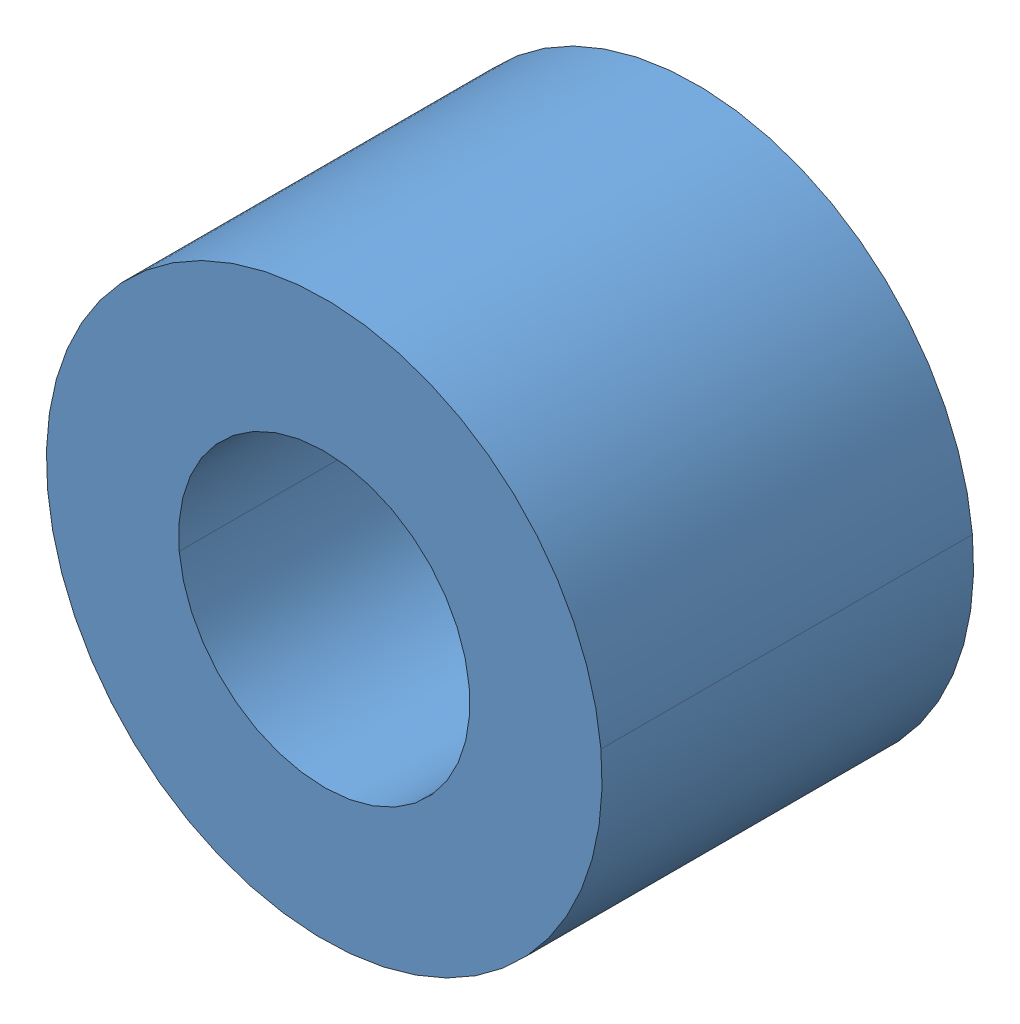
SolidWorks assembly WCP - GreyT Elevator (Cascade, 2 Stage) (1).step, configuration Default. Lengths in mm. (continued)
Components (placement in the parent): (continued)
- WCP-0326 Rev1.step-1: WCP-0326 Rev1.step [Default] at (165.1 1168.4 27.7749) x (0.127192 0.991878 0) z (0.991878 -0.127192 0) size (11.02 4.76 11) (hidden)
- WCP-0326 Rev1.step-2: WCP-0326 Rev1.step [Default] at (165.1 1193.8 27.7749) x (0.127192 0.991878 0) z (0.991878 -0.127192 0) size (11.02 4.76 11) (hidden)
- 10-32 BHCS - No Thread_WCP-0257 - 1.500.step-1: 10-32 BHCS - No Thread_WCP-0257 - 1.500.step [Default] at (101.6 1168.4 -101.6) x (-0.802481 0.596678 0) z (-0.596678 -0.802481 0) size (9.17 40.67 9.17) (hidden)
- 10-32 BHCS - No Thread_WCP-0257 - 1.500.step-2: 10-32 BHCS - No Thread_WCP-0257 - 1.500.step [Default] at (101.6 1193.8 -101.6) x (-0.802481 0.596678 0) z (-0.596678 -0.802481 0) size (9.17 40.67 9.17) (hidden)
- 10-32 BHCS - No Thread_WCP-0257 - 1.500.step-3: 10-32 BHCS - No Thread_WCP-0257 - 1.500.step [Default] at (76.2 1193.8 -101.6) x (-0.802481 0.596678 0) z (-0.596678 -0.802481 0) size (9.17 40.67 9.17) (hidden)
- 10-32 BHCS - No Thread_WCP-0257 - 1.500.step-4: 10-32 BHCS - No Thread_WCP-0257 - 1.500.step [Default] at (76.2 1168.4 -101.6) x (-0.802481 0.596678 0) z (-0.596678 -0.802481 0) size (9.17 40.67 9.17) (hidden)
- WCP-0326 Rev1.step-3: WCP-0326 Rev1.step [Default] at (101.6 1168.4 -67.4751) x (0.127192 0.991878 0) z (0.991878 -0.127192 0) size (11.02 4.76 11) (hidden)
- WCP-0326 Rev1.step-4: WCP-0326 Rev1.step [Default] at (101.6 1193.8 -67.4751) x (0.127192 0.991878 0) z (0.991878 -0.127192 0) size (11.02 4.76 11) (hidden)
- WCP-0326 Rev1.step-5: WCP-0326 Rev1.step [Default] at (76.2 1193.8 -67.4751) x (0.127192 0.991878 0) z (0.991878 -0.127192 0) size (11.02 4.76 11) (hidden)
- WCP-0326 Rev1.step-6: WCP-0326 Rev1.step [Default] at (76.2 1168.4 -67.4751) x (0.127192 0.991878 0) z (0.991878 -0.127192 0) size (11.02 4.76 11) (hidden)
- 10-32 BHCS - No Thread_WCP-0252 - 0.375.step-1: 10-32 BHCS - No Thread_WCP-0252 - 0.375.step [Default] at (165.1 11.1125 12.7) x (0.583861 0 0.811854) z (0.811854 0 -0.583861) size (9.17 12.1 9.17) (hidden)
- 10-32 BHCS - No Thread_WCP-0252 - 0.375.step-2: 10-32 BHCS - No Thread_WCP-0252 - 0.375.step [Default] at (165.1 11.1125 0) x (0.583861 0 0.811854) z (0.811854 0 -0.583861) size (9.17 12.1 9.17) (hidden)
- 10-32 BHCS - No Thread_WCP-0252 - 0.375.step-3: 10-32 BHCS - No Thread_WCP-0252 - 0.375.step [Default] at (165.1 11.1125 -12.7) x (0.583861 0 0.811854) z (0.811854 0 -0.583861) size (9.17 12.1 9.17) (hidden)
- 10-32 BHCS - No Thread_WCP-0252 - 0.375.step-4: 10-32 BHCS - No Thread_WCP-0252 - 0.375.step [Default] at (177.8 25.4 12.7) x (0 -0.948064 0.318079) z (0 0.318079 0.948064) size (9.17 12.1 9.17) (hidden)
- 10-32 BHCS - No Thread_WCP-0252 - 0.375.step-5: 10-32 BHCS - No Thread_WCP-0252 - 0.375.step [Default] at (177.8 25.4 0) x (0 -0.948064 0.318079) z (0 0.318079 0.948064) size (9.17 12.1 9.17) (hidden)
- 10-32 BHCS - No Thread_WCP-0252 - 0.375.step-6: 10-32 BHCS - No Thread_WCP-0252 - 0.375.step [Default] at (177.8 25.4 -12.7) x (0 -0.948064 0.318079) z (0 0.318079 0.948064) size (9.17 12.1 9.17) (hidden)
- 10-32 BHCS - No Thread_WCP-0252 - 0.375.step-7: 10-32 BHCS - No Thread_WCP-0252 - 0.375.step [Default] at (152.4 25.4 12.7) x (0 -0.983057 -0.183299) z (0 0.183299 -0.983057) size (9.17 12.1 9.17) (hidden)
- 10-32 BHCS - No Thread_WCP-0252 - 0.375.step-8: 10-32 BHCS - No Thread_WCP-0252 - 0.375.step [Default] at (152.4 25.4 0) x (0 -0.639879 0.768476) z (0 -0.768476 -0.639879) size (9.17 12.1 9.17) (hidden)
- 10-32 BHCS - No Thread_WCP-0252 - 0.375.step-9: 10-32 BHCS - No Thread_WCP-0252 - 0.375.step [Default] at (152.4 25.4 -12.7) x (0 -0.639879 0.768476) z (0 -0.768476 -0.639879) size (9.17 12.1 9.17) (hidden)
- 10-32 BHCS - No Thread_WCP-0252 - 0.375.step-10: 10-32 BHCS - No Thread_WCP-0252 - 0.375.step [Default] at (77.7875 50.8 -12.7) x (0 0.321661 0.946855) z (0 0.946855 -0.321661) size (9.17 12.1 9.17) (hidden)
- 10-32 BHCS - No Thread_WCP-0252 - 0.375.step-11: 10-32 BHCS - No Thread_WCP-0252 - 0.375.step [Default] at (77.7875 50.8 0) x (0 0.321661 0.946855) z (0 0.946855 -0.321661) size (9.17 12.1 9.17) (hidden)
- 10-32 BHCS - No Thread_WCP-0252 - 0.375.step-12: 10-32 BHCS - No Thread_WCP-0252 - 0.375.step [Default] at (77.7875 50.8 12.7) x (0 0.321661 0.946855) z (0 0.946855 -0.321661) size (9.17 12.1 9.17) (hidden)
- 10-32 BHCS - No Thread_WCP-0260 - 2.250.step-1: 10-32 BHCS - No Thread_WCP-0260 - 2.250.step [Default] at (76.2 1219.2 25.4) x (0.942963 -0.332897 0) z (-0.332897 -0.942963 0) size (9.17 59.72 9.17) (hidden)
- 10-32 BHCS - No Thread_WCP-0260 - 2.250.step-2: 10-32 BHCS - No Thread_WCP-0260 - 2.250.step [Default] at (101.6 1219.2 25.4) x (0.942963 -0.332897 0) z (-0.332897 -0.942963 0) size (9.17 59.72 9.17) (hidden)
- 10-32 BHCS - No Thread_WCP-0260 - 2.250.step-3: 10-32 BHCS - No Thread_WCP-0260 - 2.250.step [Default] at (76.2 25.4 25.4) x (0.942963 -0.332897 0) z (-0.332897 -0.942963 0) size (9.17 59.72 9.17) (hidden)
- 10-32 BHCS - No Thread_WCP-0260 - 2.250.step-4: 10-32 BHCS - No Thread_WCP-0260 - 2.250.step [Default] at (101.6 25.4 25.4) x (0.942963 -0.332897 0) z (-0.332897 -0.942963 0) size (9.17 59.72 9.17) (hidden)
- 10-32 BHCS - No Thread_WCP-0252 - 0.375.step-13: 10-32 BHCS - No Thread_WCP-0252 - 0.375.step [Default] at (63.5 50.8 25.4) x (0.796713 -0.604358 0) z (-0.604358 -0.796713 0) size (9.17 12.1 9.17) (hidden)
- 10-32 BHCS - No Thread_WCP-0252 - 0.375.step-14: 10-32 BHCS - No Thread_WCP-0252 - 0.375.step [Default] at (63.5 50.8 -25.4) x (-0.5764 -0.817168 0) z (0.817168 -0.5764 0) size (9.17 12.1 9.17) (hidden)
- 10-32 BHCS - No Thread_WCP-0252 - 0.375.step-15: 10-32 BHCS - No Thread_WCP-0252 - 0.375.step [Default] at (63.5 254 -25.4) x (-0.5764 -0.817168 0) z (0.817168 -0.5764 0) size (9.17 12.1 9.17) (hidden)
- 10-32 BHCS - No Thread_WCP-0252 - 0.375.step-16: 10-32 BHCS - No Thread_WCP-0252 - 0.375.step [Default] at (63.5 254 25.4) x (0.796713 -0.604358 0) z (-0.604358 -0.796713 0) size (9.17 12.1 9.17) (hidden)
- 10-32 BHCS - No Thread_WCP-0252 - 0.375.step-17: 10-32 BHCS - No Thread_WCP-0252 - 0.375.step [Default] at (77.7875 254 12.7) x (0 0.321661 0.946855) z (0 0.946855 -0.321661) size (9.17 12.1 9.17) (hidden)
- 10-32 BHCS - No Thread_WCP-0252 - 0.375.step-18: 10-32 BHCS - No Thread_WCP-0252 - 0.375.step [Default] at (77.7875 254 0) x (0 0.321661 0.946855) z (0 0.946855 -0.321661) size (9.17 12.1 9.17) (hidden)
- 10-32 BHCS - No Thread_WCP-0252 - 0.375.step-19: 10-32 BHCS - No Thread_WCP-0252 - 0.375.step [Default] at (77.7875 254 -12.7) x (0 0.321661 0.946855) z (0 0.946855 -0.321661) size (9.17 12.1 9.17) (hidden)
- 10-32 BHCS - No Thread_WCP-0252 - 0.375.step-20: 10-32 BHCS - No Thread_WCP-0252 - 0.375.step [Default] at (115.8875 1219.2 12.7) x (0 0.321661 0.946855) z (0 0.946855 -0.321661) size (9.17 12.1 9.17) (hidden)
- 10-32 BHCS - No Thread_WCP-0252 - 0.375.step-21: 10-32 BHCS - No Thread_WCP-0252 - 0.375.step [Default] at (115.8875 1219.2 0) x (0 0.321661 0.946855) z (0 0.946855 -0.321661) size (9.17 12.1 9.17) (hidden)
- 10-32 BHCS - No Thread_WCP-0252 - 0.375.step-22: 10-32 BHCS - No Thread_WCP-0252 - 0.375.step [Default] at (115.8875 1219.2 -12.7) x (0 0.321661 0.946855) z (0 0.946855 -0.321661) size (9.17 12.1 9.17) (hidden)
- 10-32 BHCS - No Thread_WCP-0252 - 0.375.step-23: 10-32 BHCS - No Thread_WCP-0252 - 0.375.step [Default] at (115.8875 25.4 -12.7) x (0 0.321661 0.946855) z (0 0.946855 -0.321661) size (9.17 12.1 9.17) (hidden)
- 10-32 BHCS - No Thread_WCP-0252 - 0.375.step-24: 10-32 BHCS - No Thread_WCP-0252 - 0.375.step [Default] at (115.8875 25.4 12.7) x (0 0.321661 0.946855) z (0 0.946855 -0.321661) size (9.17 12.1 9.17) (hidden)
- 10-32 BHCS - No Thread_WCP-0252 - 0.375.step-25: 10-32 BHCS - No Thread_WCP-0252 - 0.375.step [Default] at (115.8875 25.4 0) x (0 0.321661 0.946855) z (0 0.946855 -0.321661) size (9.17 12.1 9.17) (hidden)
- 10-32 BHCS - No Thread_WCP-0261 - 2.500.step-9: 10-32 BHCS - No Thread_WCP-0261 - 2.500.step [Default] at (38.1 25.4 25.4) x (-0.574084 -0.818796 0) z (-0.818796 0.574084 0) size (9.17 66.07 9.17) (hidden)
- 10-32 BHCS - No Thread_WCP-0261 - 2.500.step-10: 10-32 BHCS - No Thread_WCP-0261 - 2.500.step [Default] at (-50.8 25.4 25.4) x (-0.742698 -0.669626 0) z (-0.669626 0.742698 0) size (9.17 66.07 9.17) (hidden)
- 10-32 BHCS - No Thread_WCP-0261 - 2.500.step-11: 10-32 BHCS - No Thread_WCP-0261 - 2.500.step [Default] at (-38.1 25.4 25.4) x (-0.574084 -0.818796 0) z (-0.818796 0.574084 0) size (9.17 66.07 9.17) (hidden)
- 10-32 BHCS - No Thread_WCP-0261 - 2.500.step-12: 10-32 BHCS - No Thread_WCP-0261 - 2.500.step [Default] at (-25.4 25.4 25.4) x (-0.677804 -0.735243 0) z (-0.735243 0.677804 0) size (9.17 66.07 9.17) (hidden)
- WCP-0326 Rev1.step-7: WCP-0326 Rev1.step [Default] at (38.1 25.4 -31.7749) x (-0.281999 0.959415 0) z (-0.959415 -0.281999 0) size (11.02 4.76 11) (hidden)
- WCP-0326 Rev1.step-8: WCP-0326 Rev1.step [Default] at (12.7 25.4 -31.7749) x (-0.281999 0.959415 0) z (-0.959415 -0.281999 0) size (11.02 4.76 11) (hidden)
- WCP-0326 Rev1.step-9: WCP-0326 Rev1.step [Default] at (-25.4 25.4 -31.7749) x (-0.281999 0.959415 0) z (-0.959415 -0.281999 0) size (11.02 4.76 11) (hidden)
- WCP-0326 Rev1.step-10: WCP-0326 Rev1.step [Default] at (-38.1 25.4 -31.7749) x (-0.281999 0.959415 0) z (-0.959415 -0.281999 0) size (11.02 4.76 11) (hidden)
- WCP-0326 Rev1.step-11: WCP-0326 Rev1.step [Default] at (-50.8 25.4 -31.7749) x (-0.281999 0.959415 0) z (-0.959415 -0.281999 0) size (11.02 4.76 11) (hidden)
- WCP-0326 Rev1.step-12: WCP-0326 Rev1.step [Default] at (25.4 25.4 -31.7749) x (-0.281999 0.959415 0) z (-0.959415 -0.281999 0) size (11.02 4.76 11) (hidden)
- 10-32 BHCS - No Thread_WCP-0253 - 0.500.step-1: 10-32 BHCS - No Thread_WCP-0253 - 0.500.step [Default] at (-38.1 -25.4 23.114) x (0.542223 -0.840234 0) z (0.840234 0.542223 0) size (9.17 15.27 9.17) (hidden)
- 10-32 BHCS - No Thread_WCP-0253 - 0.500.step-2: 10-32 BHCS - No Thread_WCP-0253 - 0.500.step [Default] at (-12.7 -25.4 23.114) x (0.823635 -0.56712 0) z (0.56712 0.823635 0) size (9.17 15.27 9.17) (hidden)
- 10-32 BHCS - No Thread_WCP-0252 - 0.375.step-26: 10-32 BHCS - No Thread_WCP-0252 - 0.375.step [Default] at (-12.7 -11.1125 12.7) x (0.458328 0 0.888783) z (-0.888783 0 0.458328) size (9.17 12.1 9.17) (hidden)
- 10-32 BHCS - No Thread_WCP-0252 - 0.375.step-27: 10-32 BHCS - No Thread_WCP-0252 - 0.375.step [Default] at (-38.1 -11.1125 12.7) x (0.458328 0 0.888783) z (-0.888783 0 0.458328) size (9.17 12.1 9.17) (hidden)
- WCP-0326 Rev1.step-13: WCP-0326 Rev1.step [Default] at (-12.7 -17.3609 12.7) x (-0.884394 0 -0.466741) z (-0.466741 0 0.884394) size (11.02 4.76 11) (hidden)
- WCP-0326 Rev1.step-14: WCP-0326 Rev1.step [Default] at (-38.1 -17.3609 12.7) x (-0.806355 0 -0.591432) z (-0.591432 0 0.806355) size (11.02 4.76 11) (hidden)
- 10-32 BHCS - No Thread_WCP-0252 - 0.375.step-28: 10-32 BHCS - No Thread_WCP-0252 - 0.375.step [Default] at (165.1 25.4 25.4) x (0.238233 -0.971208 0) z (-0.971208 -0.238233 0) size (9.17 12.1 9.17) (hidden)
- 10-32 BHCS - No Thread_WCP-0252 - 0.375.step-29: 10-32 BHCS - No Thread_WCP-0252 - 0.375.step [Default] at (165.1 25.4 -25.4) x (0.705419 -0.708791 0) z (0.708791 0.705419 0) size (9.17 12.1 9.17) (hidden)
- #4-40 x .750L SHCS.step-1: #4-40 x .750L SHCS.step [Default] at (-4.1026 57.15 -50.8) x (0 0.222099 -0.975024) z (1 0 0) size (4.65 4.65 21.9) (hidden)
- NFS-0016_#4-40_thin_locknut_Default_As Machined_.step-1: NFS-0016_#4-40_thin_locknut_Default_As Machined_.step [Default] at (-10.35 57.15 -50.8) x (0 0.495484 -0.868617) z (0 0.868617 0.495484) size (6.37 2.79 7.35) (hidden)
- #4-40 x .750L SHCS.step-2: #4-40 x .750L SHCS.step [Default] at (-4.1026 31.75 -50.8) x (0 0.423366 0.905959) z (1 0 0) size (4.65 4.65 21.9) (hidden)
- #4-40 x .750L SHCS.step-3: #4-40 x .750L SHCS.step [Default] at (-4.1026 44.45 -50.8) x (0 -0.973772 0.227524) z (1 0 0) size (4.65 4.65 21.9) (hidden)
- NFS-0016_#4-40_thin_locknut_Default_As Machined_.step-2: NFS-0016_#4-40_thin_locknut_Default_As Machined_.step [Default] at (-10.35 44.45 -50.8) x (0 -0.910503 -0.413502) z (0 0.413502 -0.910503) size (6.37 2.79 7.35) (hidden)
- NFS-0016_#4-40_thin_locknut_Default_As Machined_.step-3: NFS-0016_#4-40_thin_locknut_Default_As Machined_.step [Default] at (-10.35 31.75 -50.8) x (0 0.495484 -0.868617) z (0 0.868617 0.495484) size (6.37 2.79 7.35) (hidden)
- 10-32 BHCS - No Thread_WCP-0261 - 2.500.step-13: 10-32 BHCS - No Thread_WCP-0261 - 2.500.step [Default] at (25.4 25.4 25.4) x (-0.992821 -0.119607 0) z (-0.119607 0.992821 0) size (9.17 66.07 9.17) (hidden)
- 10-32 BHCS - No Thread_WCP-0261 - 2.500.step-14: 10-32 BHCS - No Thread_WCP-0261 - 2.500.step [Default] at (12.7 25.4 25.4) x (-0.574084 -0.818796 0) z (-0.818796 0.574084 0) size (9.17 66.07 9.17) (hidden)
- 10-32 BHCS - No Thread_WCP-0263 - 3.000.step-1: 10-32 BHCS - No Thread_WCP-0263 - 3.000.step [Default] at (0 0 -38.1) x (0.756715 -0.653745 0) z (0.653745 0.756715 0) size (9.17 78.77 9.17) (hidden)
- 10-32 BHCS - No Thread_WCP-0263 - 3.000.step-2: 10-32 BHCS - No Thread_WCP-0263 - 3.000.step [Default] at (-50.8 0 -38.1) x (0.756715 -0.653745 0) z (0.653745 0.756715 0) size (9.17 78.77 9.17) (hidden)
- WCP-0571 Rev1.step-1: WCP-0571 Rev1.step [Default] at (-25.4 1181.1 -43.0403) size (15.88 15.88 15.71) (hidden)
- WCP-0571 Rev1.step-2: WCP-0571 Rev1.step [Default] at (-25.4 1181.1 -112.5347) x (-0.990411 -0.138152 0) z (0 0 -1) size (15.88 15.88 15.71) (hidden)
- 10-32 BHCS - No Thread_WCP-0257 - 1.500.step-5: 10-32 BHCS - No Thread_WCP-0257 - 1.500.step [Default] at (0 1181.1 -107.95) x (-0.802481 0.596678 0) z (-0.596678 -0.802481 0) size (9.17 40.67 9.17) (hidden)
- 10-32 BHCS - No Thread_WCP-0257 - 1.500.step-6: 10-32 BHCS - No Thread_WCP-0257 - 1.500.step [Default] at (-50.8 1181.1 -107.95) x (-0.853188 0.521603 0) z (-0.521603 -0.853188 0) size (9.17 40.67 9.17) (hidden)
- WCP-0560 Rev1.step-1: WCP-0560 Rev1.step [Default] at (-25.4 0 -50.8) x (-0.531612 0.846988 0) z (0 0 -1) size (47.96 47.68 9.53) (hidden)
- WCP-0560 Rev1.step-2: WCP-0560 Rev1.step [Default] at (-25.4 1181.1 -50.8) x (-0.820978 -0.57096 0) z (0 0 -1) size (47.96 47.68 9.53) (hidden)
- WCP-0583-023 Rev1.step-1: WCP-0583-023 Rev1.step [Default] at (-25.4 590.55 -50.8) x (-1 0 0) z (0 0 -1) size (50.36 1231.46 9) (hidden)
- 10-32 BHCS - No Thread_WCP-0261 - 2.500.step-15: 10-32 BHCS - No Thread_WCP-0261 - 2.500.step [Default] at (-165.1 1155.7 -30.1625) x (0.802481 0.596678 0) z (-0.596678 0.802481 0) size (9.17 66.07 9.17) (hidden)
- 10-32 BHCS - No Thread_WCP-0261 - 2.500.step-16: 10-32 BHCS - No Thread_WCP-0261 - 2.500.step [Default] at (-165.1 1143 30.1625) x (-0.999937 0.011255 0) z (0.011255 0.999937 0) size (9.17 66.07 9.17) (hidden)
- WCP-EX-0019-008.step-1: WCP-EX-0019-008.step [Default] at (88.9 31.75 -50.8) size (3 1228.38 34.58) (hidden)
- WCP-0583-015 Rev1.step-1: WCP-0583-015 Rev1.step [Default] at (88.9 1181.1 -73.025) size (34.92 38.1 6.35) (hidden)
- WCP-0476 Rev1.step-1: WCP-0476 Rev1.step [Default] at (-25.4 0 -34.925) size (63.5 34.92 6.35) (hidden)
- WCP-0476 Rev1.step-2: WCP-0476 Rev1.step [Default] at (-25.4 1181.1 -73.025) size (63.5 34.92 6.35) (hidden)
- WCP-0476 Rev1.step-3: WCP-0476 Rev1.step [Default] at (-25.4 1181.1 -104.775) size (63.5 34.92 6.35) (hidden)
- WCP-0583-025 Rev1_DefaultSM-FLAT-PATTERN.step-1: WCP-0583-025 Rev1_DefaultSM-FLAT-PATTERN.step [Default] at (22.225 25.4 -29.4) x (-1 0 0) z (0 0 -1) size (44.45 50.8 31.75) (hidden)
- WCP-0583-026 Rev1.step-1: WCP-0583-026 Rev1.step [Default] at (-31.75 25.4 -29.4) x (-1 0 0) z (0 0 -1) size (50.8 50.8 31.75) (hidden)
- WCP-0207 Rev1.step-1: WCP-0207 Rev1.step [Default] at (165.1 1193.8 -50.8) x (0 0 -1) z (0.999873 -0.015939 0) size (50.8 9.5 9.5) (hidden)
- WCP-0207 Rev1.step-2: WCP-0207 Rev1.step [Default] at (165.1 1168.4 -50.8) x (0 0 -1) z (0.999873 -0.015939 0) size (50.8 9.5 9.5) (hidden)
- WCP-0308 Rev1.step-1: WCP-0308 Rev1.step [Default] at (-50.8 0 -28.575) x (0 0 -1) z (0.995626 0.093431 0) size (6.35 9.5 9.5)
- WCP-0308 Rev1.step-2: WCP-0308 Rev1.step [Default] at (0 0 -28.575) x (0 0 -1) z (0.995626 0.093431 0) size (6.35 9.5 9.5) (hidden)
- WCP-0307 Rev1.step-1: WCP-0307 Rev1.step [Default] at (-12.7 -25.4 26.9913) x (0 0 1) z (-0.952187 0.305516 0) size (3.18 9.5 9.5) (hidden)
- WCP-0307 Rev1.step-2: WCP-0307 Rev1.step [Default] at (-38.1 -25.4 26.9913) x (0 0 1) z (-0.952187 0.305516 0) size (3.18 9.5 9.5) (hidden)
- WCP-0307 Rev1.step-3: WCP-0307 Rev1.step [Default] at (0 0 26.9913) x (0 0 1) z (-0.952187 0.305516 0) size (3.18 9.5 9.5) (hidden)
- WCP-0307 Rev1.step-4: WCP-0307 Rev1.step [Default] at (-50.8 0 26.9913) x (0 0 1) z (-0.952187 0.305516 0) size (3.18 9.5 9.5) (hidden)
- WCP-0599 Rev1.step-1: WCP-0599 Rev1.step [Default] at (-25.4 1181.1 -77.7875) x (0 0 -1) z (0.982361 -0.186992 0) size (63.5 12.67 13.72) (hidden)
- WCP-0790_500L_500_hex.step-1: WCP-0790_500L_500_hex.step [Default] at (-25.4 1181.1 -61.9125) x (0.991671 -0.128795 0) z (0 0 1) size (19.5 19.5 12.7) (hidden)
- WCP-0789_250L_500_hex.step-1: WCP-0789_250L_500_hex.step [Default] at (-25.4 0 -42.8625) size (19.5 19.5 6.35) (hidden)
- 10-32 BHCS - No Thread_WCP-0261 - 2.500.step-17: 10-32 BHCS - No Thread_WCP-0261 - 2.500.step [Default] at (-127 63.5 30.1625) x (-0.985295 -0.170861 0) z (-0.170861 0.985295 0) size (9.17 66.07 9.17) (hidden)
- 10-32 BHCS - No Thread_WCP-0261 - 2.500.step-18: 10-32 BHCS - No Thread_WCP-0261 - 2.500.step [Default] at (-127 50.8 -30.1625) x (0.742242 0.670132 0) z (-0.670132 0.742242 0) size (9.17 66.07 9.17) (hidden)
- WCP-0374 Rev1.step-1: WCP-0374 Rev1.step [Default] at (165.1 22.225 0) x (0 0 -1) z (1 0 0) size (44.07 19.05 18.67) (hidden)
- WCP-0379 Rev1.step-1: WCP-0379 Rev1.step [Default] at (165.1 22.225 0) x (0 0 -1) z (1 0 0) size (47.24 20.64 21.84) (hidden)
- WCP-0379 Rev1.step-2: WCP-0379 Rev1.step [Default] at (66.675 50.8 0) x (0 0 -1) z (0 1 0) size (47.24 20.64 21.84) (hidden)
- WCP-0374 Rev1.step-2: WCP-0374 Rev1.step [Default] at (66.675 50.8 0) x (0 0 -1) z (0 1 0) size (44.07 19.05 18.67) (hidden)
- WCP-0374 Rev1.step-3: WCP-0374 Rev1.step [Default] at (66.675 254 0) x (0 0 -1) z (0 1 0) size (44.07 19.05 18.67) (hidden)
- WCP-0379 Rev1.step-3: WCP-0379 Rev1.step [Default] at (66.675 254 0) x (0 0 -1) z (0 1 0) size (47.24 20.64 21.84) (hidden)
- WCP-0374 Rev1.step-4: WCP-0374 Rev1.step [Default] at (104.775 1219.2 0) x (0 0 -1) z (0 1 0) size (44.07 19.05 18.67) (hidden)
- WCP-0379 Rev1.step-4: WCP-0379 Rev1.step [Default] at (104.775 1219.2 0) x (0 0 -1) z (0 1 0) size (47.24 20.64 21.84) (hidden)
- WCP-0379 Rev1.step-5: WCP-0379 Rev1.step [Default] at (104.775 25.4 0) x (0 0 -1) z (0 1 0) size (47.24 20.64 21.84) (hidden)
- WCP-0374 Rev1.step-5: WCP-0374 Rev1.step [Default] at (104.775 25.4 0) x (0 0 -1) z (0 1 0) size (44.07 19.05 18.67) (hidden)
- WCP-0785_0_500_flanged_thunderhex_bearing.step-1: WCP-0785_0_500_flanged_thunderhex_bearing.step [Default] at (-25.4 0 -35.7188) x (-0.952019 0.30604 0) z (0 0 -1) size (31.12 31.12 7.94) (hidden)
- WCP-0785_0_500_flanged_thunderhex_bearing.step-2: WCP-0785_0_500_flanged_thunderhex_bearing.step [Default] at (-25.4 1181.1 -105.5688) x (-0.914179 0.405311 0) z (0 0 -1) size (31.12 31.12 7.94) (hidden)
- WCP-0785_0_500_flanged_thunderhex_bearing.step-3: WCP-0785_0_500_flanged_thunderhex_bearing.step [Default] at (-25.4 1181.1 -72.2313) x (0.656952 0.753932 0) z (0 0 1) size (31.12 31.12 7.94) (hidden)
- WCP-0800_500_hex_collar_high_strength.step-1: WCP-0800_500_hex_collar_high_strength.step [Default] at (-25.4 0 -60.325) size (28.56 28.57 9.53) (hidden)
- 10-32 BHCS - No Thread_WCP-0261 - 2.500.step-19: 10-32 BHCS - No Thread_WCP-0261 - 2.500.step [Default] at (-88.9 76.2 -30.1625) x (0.742242 0.670132 0) z (-0.670132 0.742242 0) size (9.17 66.07 9.17) (hidden)
- 10-32 BHCS - No Thread_WCP-0261 - 2.500.step-20: 10-32 BHCS - No Thread_WCP-0261 - 2.500.step [Default] at (-88.9 88.9 30.1625) x (-0.985295 -0.170861 0) z (-0.170861 0.985295 0) size (9.17 66.07 9.17) (hidden)
- 10-32 BHCS - No Thread_WCP-0261 - 2.500.step-21: 10-32 BHCS - No Thread_WCP-0261 - 2.500.step [Default] at (-88.9 228.6 30.1625) x (-0.985295 -0.170861 0) z (-0.170861 0.985295 0) size (9.17 66.07 9.17) (hidden)
- 10-32 BHCS - No Thread_WCP-0261 - 2.500.step-22: 10-32 BHCS - No Thread_WCP-0261 - 2.500.step [Default] at (-88.9 215.9 -30.1625) x (0.742242 0.670132 0) z (-0.670132 0.742242 0) size (9.17 66.07 9.17) (hidden)
- WCP-EX-0019-008.step-2: WCP-EX-0019-008.step [Default] at (-88.9 31.75 -50.8) size (3 1228.38 34.58) (hidden)
- WCP-0583-015 Rev1.step-2: WCP-0583-015 Rev1.step [Default] at (-88.9 1181.1 -73.025) x (-1 0 0) z (0 0 -1) size (34.92 38.1 6.35) (hidden)
- WCP-0326 Rev1.step-15: WCP-0326 Rev1.step [Default] at (-165.1 1193.8 27.7749) x (-0.127192 0.991878 0) z (0.991878 0.127192 0) size (11.02 4.76 11) (hidden)
- 10-32 SHCS - No Thread_WCP-0274 - 4.500.step-3: 10-32 SHCS - No Thread_WCP-0274 - 4.500.step [Default] at (-165.1 1193.8 -77.7875) x (-0.495006 -0.86889 0) z (0.86889 -0.495006 0) size (7.67 119.13 7.67) (hidden)
- WCP-0326 Rev1.step-16: WCP-0326 Rev1.step [Default] at (-165.1 1168.4 27.7749) x (-0.127192 0.991878 0) z (0.991878 0.127192 0) size (11.02 4.76 11) (hidden)
- 10-32 SHCS - No Thread_WCP-0274 - 4.500.step-4: 10-32 SHCS - No Thread_WCP-0274 - 4.500.step [Default] at (-165.1 1168.4 -77.7875) x (-0.495006 -0.86889 0) z (0.86889 -0.495006 0) size (7.67 119.13 7.67) (hidden)
- 10-32 BHCS - No Thread_WCP-0257 - 1.500.step-7: 10-32 BHCS - No Thread_WCP-0257 - 1.500.step [Default] at (-101.6 1193.8 -101.6) x (0.802481 0.596678 0) z (-0.596678 0.802481 0) size (9.17 40.67 9.17) (hidden)
- WCP-0326 Rev1.step-17: WCP-0326 Rev1.step [Default] at (-101.6 1193.8 -67.4751) x (-0.127192 0.991878 0) z (0.991878 0.127192 0) size (11.02 4.76 11) (hidden)
- 10-32 BHCS - No Thread_WCP-0257 - 1.500.step-8: 10-32 BHCS - No Thread_WCP-0257 - 1.500.step [Default] at (-101.6 1168.4 -101.6) x (0.802481 0.596678 0) z (-0.596678 0.802481 0) size (9.17 40.67 9.17) (hidden)
- WCP-0326 Rev1.step-18: WCP-0326 Rev1.step [Default] at (-101.6 1168.4 -67.4751) x (-0.127192 0.991878 0) z (0.991878 0.127192 0) size (11.02 4.76 11) (hidden)
- WCP-0326 Rev1.step-19: WCP-0326 Rev1.step [Default] at (-76.2 1168.4 -67.4751) x (-0.127192 0.991878 0) z (0.991878 0.127192 0) size (11.02 4.76 11) (hidden)
- 10-32 BHCS - No Thread_WCP-0257 - 1.500.step-9: 10-32 BHCS - No Thread_WCP-0257 - 1.500.step [Default] at (-76.2 1168.4 -101.6) x (0.802481 0.596678 0) z (-0.596678 0.802481 0) size (9.17 40.67 9.17) (hidden)
- 10-32 BHCS - No Thread_WCP-0257 - 1.500.step-10: 10-32 BHCS - No Thread_WCP-0257 - 1.500.step [Default] at (-76.2 1193.8 -101.6) x (0.802481 0.596678 0) z (-0.596678 0.802481 0) size (9.17 40.67 9.17) (hidden)
- WCP-0326 Rev1.step-20: WCP-0326 Rev1.step [Default] at (-76.2 1193.8 -67.4751) x (-0.127192 0.991878 0) z (0.991878 0.127192 0) size (11.02 4.76 11) (hidden)
- 10-32 BHCS - No Thread_WCP-0260 - 2.250.step-5: 10-32 BHCS - No Thread_WCP-0260 - 2.250.step [Default] at (-101.6 25.4 25.4) x (-0.942963 -0.332897 0) z (-0.332897 0.942963 0) size (9.17 59.72 9.17) (hidden)
- 10-32 BHCS - No Thread_WCP-0260 - 2.250.step-6: 10-32 BHCS - No Thread_WCP-0260 - 2.250.step [Default] at (-76.2 25.4 25.4) x (-0.942963 -0.332897 0) z (-0.332897 0.942963 0) size (9.17 59.72 9.17) (hidden)
- 10-32 BHCS - No Thread_WCP-0252 - 0.375.step-30: 10-32 BHCS - No Thread_WCP-0252 - 0.375.step [Default] at (-63.5 50.8 25.4) x (-0.796713 -0.604358 0) z (-0.604358 0.796713 0) size (9.17 12.1 9.17) (hidden)
- WCP-0379 Rev1.step-6: WCP-0379 Rev1.step [Default] at (-104.775 25.4 0) x (0 0 -1) z (0 -1 0) size (47.24 20.64 21.84) (hidden)
- WCP-0374 Rev1.step-6: WCP-0374 Rev1.step [Default] at (-104.775 25.4 0) x (0 0 -1) z (0 -1 0) size (44.07 19.05 18.67) (hidden)
- 10-32 BHCS - No Thread_WCP-0252 - 0.375.step-31: 10-32 BHCS - No Thread_WCP-0252 - 0.375.step [Default] at (-115.8875 25.4 0) x (0 0.321661 0.946855) z (0 -0.946855 0.321661) size (9.17 12.1 9.17) (hidden)
- 10-32 BHCS - No Thread_WCP-0252 - 0.375.step-32: 10-32 BHCS - No Thread_WCP-0252 - 0.375.step [Default] at (-115.8875 25.4 -12.7) x (0 0.321661 0.946855) z (0 -0.946855 0.321661) size (9.17 12.1 9.17) (hidden)
- 10-32 BHCS - No Thread_WCP-0252 - 0.375.step-33: 10-32 BHCS - No Thread_WCP-0252 - 0.375.step [Default] at (-115.8875 25.4 12.7) x (0 0.321661 0.946855) z (0 -0.946855 0.321661) size (9.17 12.1 9.17) (hidden)
- 10-32 BHCS - No Thread_WCP-0252 - 0.375.step-34: 10-32 BHCS - No Thread_WCP-0252 - 0.375.step [Default] at (-77.7875 50.8 0) x (0 0.321661 0.946855) z (0 -0.946855 0.321661) size (9.17 12.1 9.17) (hidden)
- 10-32 BHCS - No Thread_WCP-0252 - 0.375.step-35: 10-32 BHCS - No Thread_WCP-0252 - 0.375.step [Default] at (-77.7875 50.8 12.7) x (0 0.321661 0.946855) z (0 -0.946855 0.321661) size (9.17 12.1 9.17) (hidden)
- 10-32 BHCS - No Thread_WCP-0252 - 0.375.step-36: 10-32 BHCS - No Thread_WCP-0252 - 0.375.step [Default] at (-77.7875 50.8 -12.7) x (0 0.321661 0.946855) z (0 -0.946855 0.321661) size (9.17 12.1 9.17) (hidden)
- 10-32 BHCS - No Thread_WCP-0252 - 0.375.step-37: 10-32 BHCS - No Thread_WCP-0252 - 0.375.step [Default] at (-63.5 50.8 -25.4) x (0.5764 -0.817168 0) z (0.817168 0.5764 0) size (9.17 12.1 9.17) (hidden)
- 10-32 BHCS - No Thread_WCP-0252 - 0.375.step-38: 10-32 BHCS - No Thread_WCP-0252 - 0.375.step [Default] at (-177.8 25.4 12.7) x (0 -0.948064 0.318079) z (0 -0.318079 -0.948064) size (9.17 12.1 9.17) (hidden)
- 10-32 BHCS - No Thread_WCP-0252 - 0.375.step-39: 10-32 BHCS - No Thread_WCP-0252 - 0.375.step [Default] at (-177.8 25.4 0) x (0 -0.948064 0.318079) z (0 -0.318079 -0.948064) size (9.17 12.1 9.17) (hidden)
- 10-32 BHCS - No Thread_WCP-0252 - 0.375.step-40: 10-32 BHCS - No Thread_WCP-0252 - 0.375.step [Default] at (-177.8 25.4 -12.7) x (0 -0.948064 0.318079) z (0 -0.318079 -0.948064) size (9.17 12.1 9.17) (hidden)
- 10-32 BHCS - No Thread_WCP-0252 - 0.375.step-41: 10-32 BHCS - No Thread_WCP-0252 - 0.375.step [Default] at (-152.4 25.4 12.7) x (0 -0.983057 -0.183299) z (0 -0.183299 0.983057) size (9.17 12.1 9.17) (hidden)
- 10-32 BHCS - No Thread_WCP-0252 - 0.375.step-42: 10-32 BHCS - No Thread_WCP-0252 - 0.375.step [Default] at (-152.4 25.4 0) x (0 -0.639879 0.768476) z (0 0.768476 0.639879) size (9.17 12.1 9.17) (hidden)
- 10-32 BHCS - No Thread_WCP-0252 - 0.375.step-43: 10-32 BHCS - No Thread_WCP-0252 - 0.375.step [Default] at (-152.4 25.4 -12.7) x (0 -0.639879 0.768476) z (0 0.768476 0.639879) size (9.17 12.1 9.17) (hidden)
- WCP-0379 Rev1.step-7: WCP-0379 Rev1.step [Default] at (-165.1 22.225 0) x (0 0 -1) z (1 0 0) size (47.24 20.64 21.84) (hidden)
- WCP-0374 Rev1.step-7: WCP-0374 Rev1.step [Default] at (-165.1 22.225 0) x (0 0 -1) z (1 0 0) size (44.07 19.05 18.67) (hidden)
- 10-32 BHCS - No Thread_WCP-0252 - 0.375.step-44: 10-32 BHCS - No Thread_WCP-0252 - 0.375.step [Default] at (-165.1 11.1125 -12.7) x (-0.583861 0 0.811854) z (0.811854 0 0.583861) size (9.17 12.1 9.17) (hidden)
- 10-32 BHCS - No Thread_WCP-0252 - 0.375.step-45: 10-32 BHCS - No Thread_WCP-0252 - 0.375.step [Default] at (-165.1 11.1125 0) x (-0.583861 0 0.811854) z (0.811854 0 0.583861) size (9.17 12.1 9.17) (hidden)
- 10-32 BHCS - No Thread_WCP-0252 - 0.375.step-46: 10-32 BHCS - No Thread_WCP-0252 - 0.375.step [Default] at (-165.1 11.1125 12.7) x (-0.583861 0 0.811854) z (0.811854 0 0.583861) size (9.17 12.1 9.17) (hidden)
- 10-32 BHCS - No Thread_WCP-0252 - 0.375.step-47: 10-32 BHCS - No Thread_WCP-0252 - 0.375.step [Default] at (-63.5 254 -25.4) x (0.5764 -0.817168 0) z (0.817168 0.5764 0) size (9.17 12.1 9.17) (hidden)
- WCP-0379 Rev1.step-8: WCP-0379 Rev1.step [Default] at (-66.675 254 0) x (0 0 -1) z (0 -1 0) size (47.24 20.64 21.84) (hidden)
- WCP-0374 Rev1.step-8: WCP-0374 Rev1.step [Default] at (-66.675 254 0) x (0 0 -1) z (0 -1 0) size (44.07 19.05 18.67) (hidden)
- 10-32 BHCS - No Thread_WCP-0252 - 0.375.step-48: 10-32 BHCS - No Thread_WCP-0252 - 0.375.step [Default] at (-77.7875 254 -12.7) x (0 0.321661 0.946855) z (0 -0.946855 0.321661) size (9.17 12.1 9.17) (hidden)
- 10-32 BHCS - No Thread_WCP-0252 - 0.375.step-49: 10-32 BHCS - No Thread_WCP-0252 - 0.375.step [Default] at (-77.7875 254 0) x (0 0.321661 0.946855) z (0 -0.946855 0.321661) size (9.17 12.1 9.17) (hidden)
- 10-32 BHCS - No Thread_WCP-0252 - 0.375.step-50: 10-32 BHCS - No Thread_WCP-0252 - 0.375.step [Default] at (-77.7875 254 12.7) x (0 0.321661 0.946855) z (0 -0.946855 0.321661) size (9.17 12.1 9.17) (hidden)
- 10-32 BHCS - No Thread_WCP-0252 - 0.375.step-51: 10-32 BHCS - No Thread_WCP-0252 - 0.375.step [Default] at (-63.5 254 25.4) x (-0.796713 -0.604358 0) z (-0.604358 0.796713 0) size (9.17 12.1 9.17) (hidden)
- 10-32 BHCS - No Thread_WCP-0260 - 2.250.step-7: 10-32 BHCS - No Thread_WCP-0260 - 2.250.step [Default] at (-101.6 1219.2 25.4) x (-0.942963 -0.332897 0) z (-0.332897 0.942963 0) size (9.17 59.72 9.17) (hidden)
- 10-32 BHCS - No Thread_WCP-0260 - 2.250.step-8: 10-32 BHCS - No Thread_WCP-0260 - 2.250.step [Default] at (-76.2 1219.2 25.4) x (-0.942963 -0.332897 0) z (-0.332897 0.942963 0) size (9.17 59.72 9.17) (hidden)
- 10-32 BHCS - No Thread_WCP-0252 - 0.375.step-52: 10-32 BHCS - No Thread_WCP-0252 - 0.375.step [Default] at (-115.8875 1219.2 12.7) x (0 0.321661 0.946855) z (0 -0.946855 0.321661) size (9.17 12.1 9.17) (hidden)
- 10-32 BHCS - No Thread_WCP-0252 - 0.375.step-53: 10-32 BHCS - No Thread_WCP-0252 - 0.375.step [Default] at (-115.8875 1219.2 0) x (0 0.321661 0.946855) z (0 -0.946855 0.321661) size (9.17 12.1 9.17) (hidden)
- 10-32 BHCS - No Thread_WCP-0252 - 0.375.step-54: 10-32 BHCS - No Thread_WCP-0252 - 0.375.step [Default] at (-115.8875 1219.2 -12.7) x (0 0.321661 0.946855) z (0 -0.946855 0.321661) size (9.17 12.1 9.17) (hidden)
- WCP-0379 Rev1.step-9: WCP-0379 Rev1.step [Default] at (-104.775 1219.2 0) x (0 0 -1) z (0 -1 0) size (47.24 20.64 21.84) (hidden)
- WCP-0374 Rev1.step-9: WCP-0374 Rev1.step [Default] at (-104.775 1219.2 0) x (0 0 -1) z (0 -1 0) size (44.07 19.05 18.67) (hidden)
- WCP-0379 Rev1.step-10: WCP-0379 Rev1.step [Default] at (-66.675 50.8 0) x (0 0 -1) z (0 -1 0) size (47.24 20.64 21.84) (hidden)
- WCP-0374 Rev1.step-10: WCP-0374 Rev1.step [Default] at (-66.675 50.8 0) x (0 0 -1) z (0 -1 0) size (44.07 19.05 18.67) (hidden)
- WCP-0207 Rev1.step-3: WCP-0207 Rev1.step [Default] at (-165.1 1193.8 -50.8) x (0 0 -1) z (0.999873 0.015939 0) size (50.8 9.5 9.5) (hidden)
- WCP-0207 Rev1.step-4: WCP-0207 Rev1.step [Default] at (-165.1 1168.4 -50.8) x (0 0 -1) z (0.999873 0.015939 0) size (50.8 9.5 9.5) (hidden)
- 10-32 BHCS - No Thread_WCP-0252 - 0.375.step-55: 10-32 BHCS - No Thread_WCP-0252 - 0.375.step [Default] at (-165.1 25.4 25.4) x (-0.238233 -0.971208 0) z (-0.971208 0.238233 0) size (9.17 12.1 9.17) (hidden)
- 10-32 BHCS - No Thread_WCP-0252 - 0.375.step-56: 10-32 BHCS - No Thread_WCP-0252 - 0.375.step [Default] at (-165.1 25.4 -25.4) x (-0.705419 -0.708791 0) z (0.708791 -0.705419 0) size (9.17 12.1 9.17) (hidden)
- WCP-EX-0019-004.step-2: WCP-EX-0019-004.step [Default] at (-127 622.3 0) x (0 1 0) z (1 0 0) size (1219.2 50.8 25.4) (hidden)
- MirrorWCP-EX-0019-005.step-1: MirrorWCP-EX-0019-005.step [Default] at (-88.9 152.4 0) x (0 -1 0) z (-1 0 0) size (228.6 50.8 25.4) (hidden)
- WCP-0523 Rev1.step-1: WCP-0523 Rev1.step [Default] at (88.9 152.4 -41.6719) x (0.995786 -0.091702 0) z (-0.091702 -0.995786 0) size (15.88 0.79 15.88) (hidden)
- 10-32 BHCS - No Thread_WCP-0263 - 3.000.step-3: 10-32 BHCS - No Thread_WCP-0263 - 3.000.step [Default] at (88.9 152.4 -42.0688) x (0.163054 -0.986617 0) z (0.986617 0.163054 0) size (9.17 78.77 9.17) (hidden)
- WCP-0326 Rev1.step-21: WCP-0326 Rev1.step [Default] at (88.9 152.4 27.7749) x (0.982047 -0.188635 0) z (-0.188635 -0.982047 0) size (11.02 4.76 11) (hidden)
- WCP-0523 Rev1.step-2: WCP-0523 Rev1.step [Default] at (-88.9 152.4 -41.6719) x (0.726757 0.686895 0) z (0.686895 -0.726757 0) size (15.88 0.79 15.88) (hidden)
- WCP-0326 Rev1.step-22: WCP-0326 Rev1.step [Default] at (-88.9 152.4 27.7749) x (0.925745 -0.378148 0) z (-0.378148 -0.925745 0) size (11.02 4.76 11) (hidden)
- 10-32 BHCS - No Thread_WCP-0263 - 3.000.step-4: 10-32 BHCS - No Thread_WCP-0263 - 3.000.step [Default] at (-88.9 152.4 -42.0688) x (0.163054 -0.986617 0) z (0.986617 0.163054 0) size (9.17 78.77 9.17) (hidden)
- WCP-0203 Rev1.step-1: WCP-0203 Rev1.step [Default] at (88.9 152.4 -33.3375) x (0 0 1) z (0.991701 -0.128564 0) size (15.88 9.5 9.5) (hidden)
- WCP-0203 Rev1.step-2: WCP-0203 Rev1.step [Default] at (-88.9 152.4 -33.3375) x (0 0 1) z (-0.976351 -0.216192 0) size (15.88 9.5 9.5) (hidden)
- WCP-0583-027 Rev1.step-1: WCP-0583-027 Rev1.step [Default] at (-38.1 -12.7 25.4) x (0 -1 0) z (1 0 0) size (25.4 25.4 50.8) (hidden)
